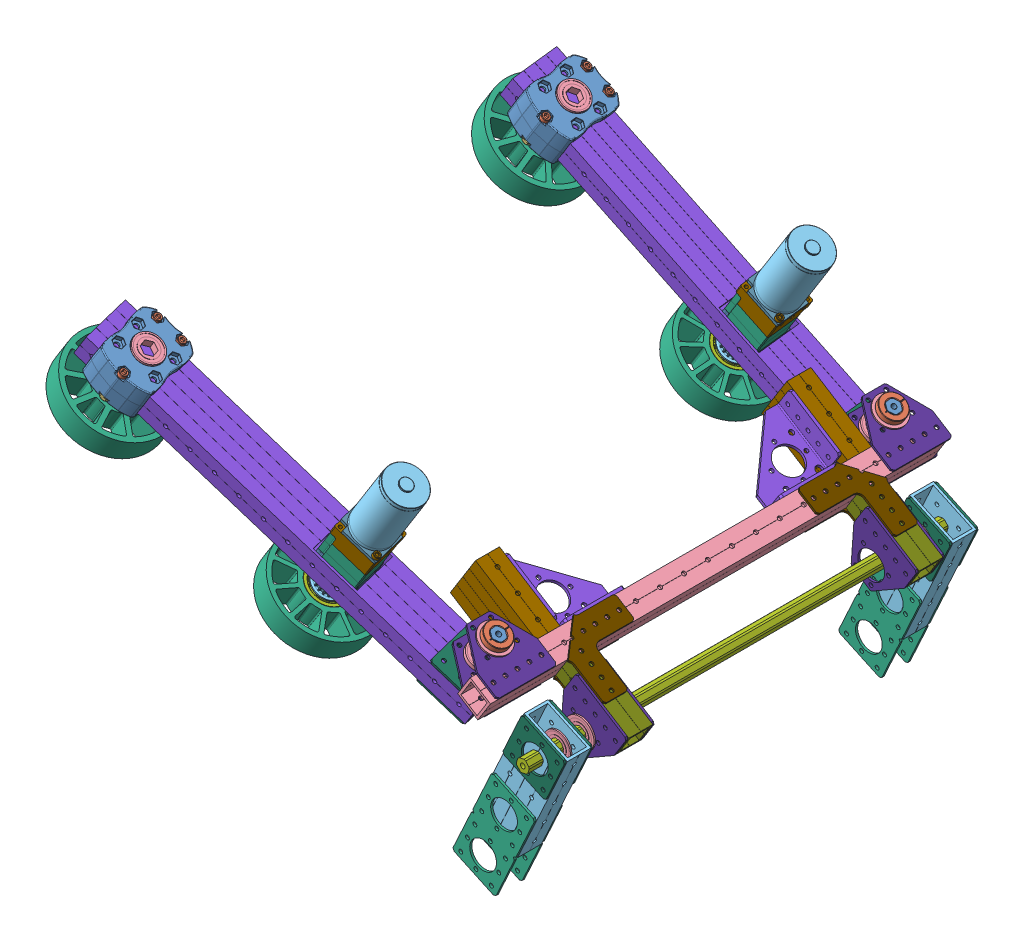
SolidWorks assembly Intake, configuration Default. Lengths in mm.
Overall size (503.07 503.81 614.92).
182 component instances, 45 part files, 124 mates.
Components (placement in the parent):
- Arm-3: Arm [Default] at (-23.47 463.3123 635.721) x (-0.531639 -0.846966 -0.002975) z (-0.831467 0.521235 0.192294) size (182.24 117.43 425.71)
  - PlasticBerringClamps-1: PlasticBerringClamps [Default] at (91.1348 153.644 -362.2083) size (41.46 73.98 53.68)
    - 217-4155-001 Rev6-1: 217-4155-001 Rev6 [Default] at (-3.3739 45.2343 730.1325) x (0 0 -1) z (1 0 0) size (53.68 71 22.06)
    - 217-4155-001 Rev6-2: 217-4155-001 Rev6 [Default] at (-3.3739 45.2343 730.1325) x (0 0 1) z (-1 0 0) size (53.68 71 22.06)
    - 217-4155-003 Rev1_SSA1032-1375ZB-1: 217-4155-003 Rev1_SSA1032-1375ZB [Default] at (-18.0739 75.1843 730.1325) x (0 1 0) z (0 0 1) size (7.87 39.75 7.87)
    - 217-4155-003 Rev1_SSA1032-1375ZB-2: 217-4155-003 Rev1_SSA1032-1375ZB [Default] at (-18.0739 15.2843 717.4325) x (0 1 0) z (0 0 1) size (7.87 39.75 7.87)
    - 217-4155-003 Rev1_SSA1032-1375ZB-3: 217-4155-003 Rev1_SSA1032-1375ZB [Default] at (-18.0739 15.2843 742.8325) x (0 1 0) z (0 0 1) size (7.87 39.75 7.87)
    - 217-4155-002 Rev2_NNY1032-ZC-1: 217-4155-002 Rev2_NNY1032-ZC [Default] at (11.3261 15.2843 717.4325) x (0 -0.5 -0.866025) z (1 0 0) size (9.39 10.84 4.45)
    - 217-4155-002 Rev2_NNY1032-ZC-2: 217-4155-002 Rev2_NNY1032-ZC [Default] at (11.3261 15.2843 742.8325) x (0 -0.5 -0.866025) z (1 0 0) size (9.39 10.84 4.45)
    - 217-4155-002 Rev2_NNY1032-ZC-3: 217-4155-002 Rev2_NNY1032-ZC [Default] at (11.3261 75.1843 730.1325) x (0 0.5 -0.866025) z (1 0 0) size (9.39 10.84 4.45)
    - FlangedBerring-1: FlangedBerring [Default] at (17.3541 43.6343 730.1325) x (0 0.579557 0.814931) z (0 -0.814931 0.579557) size (31.12 7.94 31.12)
    - FlangedBerring-2: FlangedBerring [Default] at (-24.1019 43.6343 730.1325) x (0 0.415973 -0.909377) z (0 -0.909377 -0.415973) size (31.12 7.94 31.12)
  - 18tSproket-1: 18tSproket [Default] at (115.7389 197.2783 367.9242) x (0 0.046999 0.998895) z (1 0 0) size (32 32 14.5)
  - 18tSproket-2: 18tSproket [Default] at (115.7389 199.082 150.8743) x (0 0.078751 0.996894) z (-1 0 0) size (32 32 14.5)
  - 4inTractionWheels-1: 4inTractionWheels [Default] at (129.7369 180.6221 368.9515) x (0 -0.985371 -0.170422) z (1 0 0) size (101.6 101.6 25.74)
    - 4IN Compliant Wheel FINAL Overmold-1: 4IN Compliant Wheel FINAL Overmold [Default] at (-16.2374 3.8509 18.652) size (101.6 101.6 25.74)
    - 2in Wheel Intergrated 0500 HEX Hub-1: 2in Wheel Intergrated 0500 HEX Hub [Default] at (-16.2374 3.8509 5.952) x (-1 0 0) z (0 0 -1) size (41.91 41.91 25.4)
  - 4inTractionWheels-2: 4inTractionWheels [Default] at (141.6409 215.6464 152.9003) x (0 0.993829 -0.110924) z (-1 0 0) size (101.6 101.6 25.74)
    - 4IN Compliant Wheel FINAL Overmold-1: 4IN Compliant Wheel FINAL Overmold [Default] at (-16.2374 3.8509 18.652) size (101.6 101.6 25.74)
    - 2in Wheel Intergrated 0500 HEX Hub-1: 2in Wheel Intergrated 0500 HEX Hub [Default] at (-16.2374 3.8509 5.952) x (-1 0 0) z (0 0 -1) size (41.91 41.91 25.4)
  - 1x2x16StockSlotted-1: 1x2x16StockSlotted [12] at (87.8609 198.8783 750.2323) x (-1 0 0) z (0 0 -1) size (25.4 50.8 406.4)
  - BagMotor2StageGearBox-1: BagMotor2StageGearBox [Default] at (46.4959 199.082 150.8743) x (0 0 1) z (-1 0 0) size (49.3 49.3 173.58)
    - 217-2625-001 Rev1-1: 217-2625-001 Rev1 [Default] at origin size (42 42 18)
    - 217-2625-002 Rev1-1: 217-2625-002 Rev1 [Default] at (0 0 -29.4) size (42 42 17.13)
    - 217-2625-003 Rev1-1: 217-2625-003 Rev1 [Default] at (0 0 -43.6478) x (0.966651 -0.256095 0) z (0 0 -1) size (17 17 64.12)
    - 217-2625-009 Rev1-1: 217-2625-009 Rev1 [Default] at (0 0 -3.48) x (-0.609619 0.792694 0) z (0 0 -1) size (18 18 13)
    - 217-2625-100-1: 217-2625-100 [Default] at (0 0 -18.8454) x (0.784104 -0.62063 0) z (0 0 1) size (39.26 38.9 12.7)
      - 217-2625-008 Rev1-1: 217-2625-008 Rev1 [Default] at origin size (34.7 34.7 4.7)
      - 217-2625-010 Rev1-1: 217-2625-010 Rev1 [Default] at (0 10.193 3.65) x (0.999813 0.019336 0) z (0 0 1) size (4 4 12)
      - 217-2625-010 Rev1-2: 217-2625-010 Rev1 [Default] at (8.691 -5.3258 3.65) size (4 4 12)
      - 217-2625-010 Rev1-3: 217-2625-010 Rev1 [Default] at (-8.691 -5.3258 3.65) size (4 4 12)
      - 217-2625-005 Rev1_Planet_Revolving_Follower01-1: 217-2625-005 Rev1_Planet_Revolving_Follower01 [Default] at (8.691 -5.3258 6.35) x (0.932816 0.360354 0) z (0 0 1) size (16.91 16.92 8)
      - 217-2625-005 Rev1_Planet_Revolving_Follower01-2: 217-2625-005 Rev1_Planet_Revolving_Follower01 [Default] at (-8.691 -5.3258 6.35) x (-0.932788 -0.360426 0) z (0 0 1) size (16.91 16.92 8)
      - 217-2625-005 Rev1_Planet_Revolving_Follower01-3: 217-2625-005 Rev1_Planet_Revolving_Follower01 [Default] at (0 10.193 6.35) x (0.893583 0.448898 0) z (0 0 1) size (16.91 16.92 8)
    - 217-2625-007 Rev1_Sun_Driver01-1: 217-2625-007 Rev1_Sun_Driver01 [Default] at (0 0 -11.5575) x (0.564419 -0.825488 0) z (0 0 1) size (14.49 14.49 12.72)
    - 217-2742-1: 217-2742 [Default] at (0 0 -51.4002) x (0 0 1) z (-0.997393 0.072165 0) size (7 28 28)
    - 217-2742-2: 217-2742 [Default] at (0 0 -43.1002) x (0 0 1) z (-1 0 0) size (7 28 28)
    - 217-2741-1: 217-2741 [Default] at (0 0 -7) x (0 0 1) z (-0.951311 0.308231 0) size (5 26 26)
    - TRUARC-MSH-15_98541A410-1: TRUARC-MSH-15_98541A410 [Default] at (0 0 -35.4954) x (0 0 -1) z (0.980859 -0.194721 0) size (1 19.6 17.4)
    - SPRGW0856-1102-012_9714K62-1: SPRGW0856-1102-012_9714K62 [Default] at (0 0 -44.1002) x (-0.695225 0.718792 0) z (-0.718792 -0.695225 0) size (29.09 5.11 30.79)
    - SSS1032-0125ZB_94105A824-1: SSS1032-0125ZB_94105A824 [Default] at (5.4759 4.2112 1.995) x (-0.605001 0.78669 -0.122849) z (0.792694 0.609619 0) size (4.83 4.84 3.3)
    - TRUARC-5103-68_97414A675_grv-1: TRUARC-5103-68_97414A675_grv [Default] at (1.1965 0.0349 -1.3834) x (0 0 -1) z (-0.029125 0.999576 0) size (1.07 15.49 20.19)
    - 217-3351-1: 217-3351 [Default] at (0 0 10.675) x (0 -1 0) z (0 0 -1) size (40.4 40.4 81.5)
    - 217-2816-001 Rev1-1: 217-2816-001 Rev1 [Default] at (0 0 -29.55) x (1 0 0) z (0 0 -1) size (42 42 14.5)
    - SSA_SSA0832-1750ZC-1: SSA_SSA0832-1750ZC [Default] at (-17.5 17.5 -47.261) x (-0.769034 -0.639207 0) z (0.639207 -0.769034 0) size (6.73 48.51 6.73)
    - SSA_SSA0832-1750ZC-2: SSA_SSA0832-1750ZC [Default] at (17.5 -17.5 -47.261) x (0.162252 0.986749 0) z (-0.986749 0.162252 0) size (6.73 48.51 6.73)
    - 217-2625-011 Rev1-1: 217-2625-011 Rev1 [Default] at (0 0 1.37) x (-0.792694 -0.609619 0) z (-0.609619 0.792694 0) size (8.01 7.5 7.94)
    - SSA_SSA0832-0500ZC-1: SSA_SSA0832-0500ZC [Default] at (-17.5 17.5 10.675) x (0.592766 0.805375 0) z (0.805375 -0.592766 0) size (6.73 16.76 6.73)
    - SSA_SSA0832-0500ZC-2: SSA_SSA0832-0500ZC [Default] at (17.5 -17.5 10.675) x (-0.592766 -0.805375 0) z (-0.805375 0.592766 0) size (6.73 16.76 6.73)
    - SSHCM004_SSHCM004070010C-1: SSHCM004_SSHCM004070010C [Default] at (0 -12.5 7.5) x (-0.451598 -0.892221 0) z (0.892221 -0.451598 0) size (7 14 7)
    - SSHCM004_SSHCM004070010C-2: SSHCM004_SSHCM004070010C [Default] at (0 12.5 7.5) x (-0.447517 -0.894275 0) z (0.894275 -0.447517 0) size (7 14 7)
    - 217-2816-001 Rev1-2: 217-2816-001 Rev1 [Default] at (0 0 -16.85) x (1 0 0) z (0 0 -1) size (42 42 14.5)
    - 217-2818 Rev1-1: 217-2818 Rev1 [Default] at (0 0 -31.5454) size (49.07 49.07 17.4)
      - 217-2725-001 Rev1_24t Sun-1: 217-2725-001 Rev1_24t Sun [Default] at (0 0 8.7) size (14.45 14.45 12.7)
      - 217-2725-002 Rev1_24t Planet-1: 217-2725-002 Rev1_24t Planet [Default] at (-12.089 0 6.35) x (-0.130526 0.991445 0) z (0 0 -1) size (13.17 13.15 8)
      - 217-2724-002 Rev1-1: 217-2724-002 Rev1 [Default] x (0.707107 -0.707107 0) z (0 0 -1) size (34.7 34.7 4.7)
      - 217-2625-010 Rev1-1: 217-2625-010 Rev1 [Default] at (-12.089 0 3.65) x (0.971612 -0.236582 0) z (0 0 1) size (4 4 12)
      - 217-2725-002 Rev1_24t Planet-2: 217-2725-002 Rev1_24t Planet [Default] at (0 -12.089 6.35) x (-0.991445 -0.130526 0) z (0 0 -1) size (13.17 13.15 8)
      - 217-2725-002 Rev1_24t Planet-3: 217-2725-002 Rev1_24t Planet [Default] at (12.089 0 6.35) x (0.130526 -0.991445 0) z (0 0 -1) size (13.17 13.15 8)
      - 217-2725-002 Rev1_24t Planet-4: 217-2725-002 Rev1_24t Planet [Default] at (0 12.089 6.35) x (0.991445 0.130526 0) z (0 0 -1) size (13.17 13.15 8)
      - 217-2625-010 Rev1-2: 217-2625-010 Rev1 [Default] at (0 -12.089 3.65) x (0.236582 0.971612 0) z (0 0 1) size (4 4 12)
      - 217-2625-010 Rev1-3: 217-2625-010 Rev1 [Default] at (12.089 0 3.65) x (-0.971612 0.236582 0) z (0 0 1) size (4 4 12)
      - 217-2625-010 Rev1-4: 217-2625-010 Rev1 [Default] at (0 12.089 3.65) x (-0.236582 -0.971612 0) z (0 0 1) size (4 4 12)
    - 217-2822-003 Rev4-1: 217-2822-003 Rev4 [Default] at (0 0 9) x (0 -1 0) z (0 0 1) size (42 42 4.8)
  - FaceBerringMountGussetHalved-1: FaceBerringMountGussetHalved [Default] at (72.8749 224.1513 26.2053) x (0 1 0) z (1 0 0) size (50.67 50.55 2.29)
  - FaceBerringMountGussetHalved-3: FaceBerringMountGussetHalved [Default] at (100.5609 198.7513 0.9323) x (0 0 -1) z (1 0 0) size (50.67 50.55 2.29)
  - FlangedBerring-1: FlangedBerring [Default] at (96.4969 198.7513 27.6404) x (0 0.415973 -0.909377) z (0 -0.909377 -0.415973) size (31.12 7.94 31.12)
  - FlangedBerring-2: FlangedBerring [Default] at (79.2249 197.4432 26.2053) x (0 -0.140437 0.99009) z (0 -0.99009 -0.140437) size (31.12 7.94 31.12)
- 1x1x3Stock-3: 1x1x3Stock [Default] at (630.636 -4.873 778.4629) x (-0.002909 -0.001687 0.999994) z (0.846966 -0.531645 0.001567) size (25.4 25.4 76.2)
- SideBerringGusset-2: SideBerringGusset [Default] at (-31.1533 428.0283 834.4183) x (0.002909 0.001687 -0.999994) z (-0.531639 -0.846966 -0.002975) size (63.5 61.91 2.29)
- SideBerringGusset-3: SideBerringGusset [Default] at (-47.0875 402.643 834.3291) x (-0.002909 -0.001687 0.999994) z (0.531639 0.846966 0.002975) size (63.5 61.91 2.29)
- FlangedBerring-11: FlangedBerring [Default] at (-34.5292 422.6501 834.3994) x (0.844713 -0.529962 -0.07483) z (0.061802 -0.042296 0.997192) size (31.12 7.94 31.12)
- FlangedBerring-12: FlangedBerring [Default] at (-43.7116 408.0213 834.348) x (-0.292306 0.180181 0.939198) z (0.794932 -0.500184 0.343364) size (31.12 7.94 31.12)
- SideBerringGusset-4: SideBerringGusset [Default] at (19.3994 346.1992 454.4895) x (0.846966 -0.531645 0.001567) z (-0.002909 -0.001687 0.999994) size (63.5 61.91 2.29)
- FlangedBerring-13: FlangedBerring [Default] at (19.3809 346.1885 460.8395) x (0.999707 0.024044 0.002949) z (-0.024049 0.999709 0.001616) size (31.12 7.94 31.12)
- SideBerringGusset-5: SideBerringGusset [Default] at (18.4974 345.6762 764.5734) x (-0.846966 0.531645 -0.001567) z (0.002909 0.001687 -0.999994) size (63.5 61.91 2.29)
- SideBerringGusset-6: SideBerringGusset [Default] at (18.4235 345.6333 789.9733) x (0.846966 -0.531645 0.001567) z (-0.002909 -0.001687 0.999994) size (63.5 61.91 2.29)
- SideBerringGusset-7: SideBerringGusset [Default] at (19.3188 346.1525 482.1754) x (0.846966 -0.531645 0.001567) z (-0.002909 -0.001687 0.999994) size (63.5 61.91 2.29)
- FlangedBerring-15: FlangedBerring [Default] at (18.4353 345.6402 785.9093) x (-0.001685 0.999997 0.001682) z (0.999994 0.00168 0.002912) size (31.12 7.94 31.12)
- 1x1x3Stock-5: 1x1x3Stock [Default] at (631.5313 -4.3539 470.665) x (-0.002909 -0.001687 0.999994) z (0.846966 -0.531645 0.001567) size (25.4 25.4 76.2)
- PlusGussetHalved-7: PlusGussetHalved [Default] at (-22.7192 387.5477 777.2242) x (-0.846966 0.531645 -0.001567) z (0.531639 0.846966 0.002975) size (71.47 72 2.29)
- PlusGussetHalved-8: PlusGussetHalved [Default] at (-7.1049 411.5159 469.5087) x (0.002909 0.001687 -0.999994) z (0.531639 0.846966 0.002975) size (71.47 72 2.29)
- PlusGussetHalved-9: PlusGussetHalved [Default] at (-21.8239 388.0668 469.4263) x (0.002909 0.001687 -0.999994) z (0.531639 0.846966 0.002975) size (71.47 72 2.29)
- SideBerringGusset-8: SideBerringGusset [Default] at (-45.8684 403.3499 415.2315) x (-0.002909 -0.001687 0.999994) z (0.531639 0.846966 0.002975) size (63.5 61.91 2.29)
- SideBerringGusset-9: SideBerringGusset [Default] at (-31.1494 426.799 415.3138) x (-0.002909 -0.001687 0.999994) z (0.531639 0.846966 0.002975) size (63.5 61.91 2.29)
- FlangedBerring-19: FlangedBerring [Default] at (-33.31 423.3569 415.3017) x (0.837705 -0.525302 -0.149357) z (0.124937 -0.081896 0.988779) size (31.12 7.94 31.12)
- FlangedBerring-21: FlangedBerring [Default] at (-42.4925 408.7281 415.2504) x (-0.844713 0.529962 0.07483) z (0.061802 -0.042296 0.997192) size (31.12 7.94 31.12)
- HexShaft3.5in-1: HexShaft3.5in [Default] at (48.5558 553.7791 415.7599) x (-0.061802 0.042296 -0.997192) z (0.531639 0.846966 0.002975) size (13.74 12.75 88.9)
- ShaftCollar-1: ShaftCollar [Default] at (-27.4022 432.7688 415.3348) x (-0.061802 0.042296 -0.997192) z (0.531639 0.846966 0.002975) size (25.39 25.4 7.82)
- 1_4inSpacer-1: 1_4inSpacer [Default] at (-48.4003 399.3162 415.2173) x (-0.061802 0.042296 -0.997192) z (0.531639 0.846966 0.002975) size (19.5 19.5 6.35)
- ShaftCollar-2: ShaftCollar [Default] at (-70.5169 366.5607 416.5259) x (-0.061802 0.042296 -0.997192) z (0.531639 0.846966 0.002975) size (25.39 25.4 7.82)
- Arm-5: Arm [Default] at (-4.0746 452.6105 216.4592) x (-0.531639 -0.846966 -0.002975) z (-0.843997 0.529475 0.085594) size (182.24 117.43 425.71)
  - PlasticBerringClamps-1: PlasticBerringClamps [Default] at (91.1348 153.644 -362.2083) size (41.46 73.98 53.68)
    - 217-4155-001 Rev6-1: 217-4155-001 Rev6 [Default] at (-3.3739 45.2343 730.1325) x (0 0 -1) z (1 0 0) size (53.68 71 22.06)
    - 217-4155-001 Rev6-2: 217-4155-001 Rev6 [Default] at (-3.3739 45.2343 730.1325) x (0 0 1) z (-1 0 0) size (53.68 71 22.06)
    - 217-4155-003 Rev1_SSA1032-1375ZB-1: 217-4155-003 Rev1_SSA1032-1375ZB [Default] at (-18.0739 75.1843 730.1325) x (0 1 0) z (0 0 1) size (7.87 39.75 7.87)
    - 217-4155-003 Rev1_SSA1032-1375ZB-2: 217-4155-003 Rev1_SSA1032-1375ZB [Default] at (-18.0739 15.2843 717.4325) x (0 1 0) z (0 0 1) size (7.87 39.75 7.87)
    - 217-4155-003 Rev1_SSA1032-1375ZB-3: 217-4155-003 Rev1_SSA1032-1375ZB [Default] at (-18.0739 15.2843 742.8325) x (0 1 0) z (0 0 1) size (7.87 39.75 7.87)
    - 217-4155-002 Rev2_NNY1032-ZC-1: 217-4155-002 Rev2_NNY1032-ZC [Default] at (11.3261 15.2843 717.4325) x (0 -0.5 -0.866025) z (1 0 0) size (9.39 10.84 4.45)
    - 217-4155-002 Rev2_NNY1032-ZC-2: 217-4155-002 Rev2_NNY1032-ZC [Default] at (11.3261 15.2843 742.8325) x (0 -0.5 -0.866025) z (1 0 0) size (9.39 10.84 4.45)
    - 217-4155-002 Rev2_NNY1032-ZC-3: 217-4155-002 Rev2_NNY1032-ZC [Default] at (11.3261 75.1843 730.1325) x (0 0.5 -0.866025) z (1 0 0) size (9.39 10.84 4.45)
    - FlangedBerring-1: FlangedBerring [Default] at (17.3541 43.6343 730.1325) x (0 0.579557 0.814931) z (0 -0.814931 0.579557) size (31.12 7.94 31.12)
    - FlangedBerring-2: FlangedBerring [Default] at (-24.1019 43.6343 730.1325) x (0 0.415973 -0.909377) z (0 -0.909377 -0.415973) size (31.12 7.94 31.12)
  - 18tSproket-1: 18tSproket [Default] at (115.7389 197.2783 367.9242) x (0 0.046999 0.998895) z (1 0 0) size (32 32 14.5)
  - 18tSproket-2: 18tSproket [Default] at (115.7389 199.082 150.8743) x (0 0.078751 0.996894) z (-1 0 0) size (32 32 14.5)
  - 4inTractionWheels-1: 4inTractionWheels [Default] at (129.7369 180.6221 368.9515) x (0 -0.985371 -0.170422) z (1 0 0) size (101.6 101.6 25.74)
    - 4IN Compliant Wheel FINAL Overmold-1: 4IN Compliant Wheel FINAL Overmold [Default] at (-16.2374 3.8509 18.652) size (101.6 101.6 25.74)
    - 2in Wheel Intergrated 0500 HEX Hub-1: 2in Wheel Intergrated 0500 HEX Hub [Default] at (-16.2374 3.8509 5.952) x (-1 0 0) z (0 0 -1) size (41.91 41.91 25.4)
  - 4inTractionWheels-2: 4inTractionWheels [Default] at (141.6409 215.6464 152.9003) x (0 0.993829 -0.110924) z (-1 0 0) size (101.6 101.6 25.74)
    - 4IN Compliant Wheel FINAL Overmold-1: 4IN Compliant Wheel FINAL Overmold [Default] at (-16.2374 3.8509 18.652) size (101.6 101.6 25.74)
    - 2in Wheel Intergrated 0500 HEX Hub-1: 2in Wheel Intergrated 0500 HEX Hub [Default] at (-16.2374 3.8509 5.952) x (-1 0 0) z (0 0 -1) size (41.91 41.91 25.4)
  - 1x2x16StockSlotted-1: 1x2x16StockSlotted [12] at (87.8609 198.8783 750.2323) x (-1 0 0) z (0 0 -1) size (25.4 50.8 406.4)
  - BagMotor2StageGearBox-1: BagMotor2StageGearBox [Default] at (46.4959 199.082 150.8743) x (0 0 1) z (-1 0 0) size (49.3 49.3 173.58)
    - 217-2625-001 Rev1-1: 217-2625-001 Rev1 [Default] at origin size (42 42 18)
    - 217-2625-002 Rev1-1: 217-2625-002 Rev1 [Default] at (0 0 -29.4) size (42 42 17.13)
    - 217-2625-003 Rev1-1: 217-2625-003 Rev1 [Default] at (0 0 -43.6478) x (0.966651 -0.256095 0) z (0 0 -1) size (17 17 64.12)
    - 217-2625-009 Rev1-1: 217-2625-009 Rev1 [Default] at (0 0 -3.48) x (-0.609619 0.792694 0) z (0 0 -1) size (18 18 13)
    - 217-2625-100-1: 217-2625-100 [Default] at (0 0 -18.8454) x (0.784104 -0.62063 0) z (0 0 1) size (39.26 38.9 12.7)
      - 217-2625-008 Rev1-1: 217-2625-008 Rev1 [Default] at origin size (34.7 34.7 4.7)
      - 217-2625-010 Rev1-1: 217-2625-010 Rev1 [Default] at (0 10.193 3.65) x (0.999813 0.019336 0) z (0 0 1) size (4 4 12)
      - 217-2625-010 Rev1-2: 217-2625-010 Rev1 [Default] at (8.691 -5.3258 3.65) size (4 4 12)
      - 217-2625-010 Rev1-3: 217-2625-010 Rev1 [Default] at (-8.691 -5.3258 3.65) size (4 4 12)
      - 217-2625-005 Rev1_Planet_Revolving_Follower01-1: 217-2625-005 Rev1_Planet_Revolving_Follower01 [Default] at (8.691 -5.3258 6.35) x (0.932816 0.360354 0) z (0 0 1) size (16.91 16.92 8)
      - 217-2625-005 Rev1_Planet_Revolving_Follower01-2: 217-2625-005 Rev1_Planet_Revolving_Follower01 [Default] at (-8.691 -5.3258 6.35) x (-0.932788 -0.360426 0) z (0 0 1) size (16.91 16.92 8)
      - 217-2625-005 Rev1_Planet_Revolving_Follower01-3: 217-2625-005 Rev1_Planet_Revolving_Follower01 [Default] at (0 10.193 6.35) x (0.893583 0.448898 0) z (0 0 1) size (16.91 16.92 8)
    - 217-2625-007 Rev1_Sun_Driver01-1: 217-2625-007 Rev1_Sun_Driver01 [Default] at (0 0 -11.5575) x (0.564419 -0.825488 0) z (0 0 1) size (14.49 14.49 12.72)
    - 217-2742-1: 217-2742 [Default] at (0 0 -51.4002) x (0 0 1) z (-0.997393 0.072165 0) size (7 28 28)
    - 217-2742-2: 217-2742 [Default] at (0 0 -43.1002) x (0 0 1) z (-1 0 0) size (7 28 28)
    - 217-2741-1: 217-2741 [Default] at (0 0 -7) x (0 0 1) z (-0.951311 0.308231 0) size (5 26 26)
    - TRUARC-MSH-15_98541A410-1: TRUARC-MSH-15_98541A410 [Default] at (0 0 -35.4954) x (0 0 -1) z (0.980859 -0.194721 0) size (1 19.6 17.4)
    - SPRGW0856-1102-012_9714K62-1: SPRGW0856-1102-012_9714K62 [Default] at (0 0 -44.1002) x (-0.695225 0.718792 0) z (-0.718792 -0.695225 0) size (29.09 5.11 30.79)
    - SSS1032-0125ZB_94105A824-1: SSS1032-0125ZB_94105A824 [Default] at (5.4759 4.2112 1.995) x (-0.605001 0.78669 -0.122849) z (0.792694 0.609619 0) size (4.83 4.84 3.3)
    - TRUARC-5103-68_97414A675_grv-1: TRUARC-5103-68_97414A675_grv [Default] at (1.1965 0.0349 -1.3834) x (0 0 -1) z (-0.029125 0.999576 0) size (1.07 15.49 20.19)
    - 217-3351-1: 217-3351 [Default] at (0 0 10.675) x (0 -1 0) z (0 0 -1) size (40.4 40.4 81.5)
    - 217-2816-001 Rev1-1: 217-2816-001 Rev1 [Default] at (0 0 -29.55) x (1 0 0) z (0 0 -1) size (42 42 14.5)
    - SSA_SSA0832-1750ZC-1: SSA_SSA0832-1750ZC [Default] at (-17.5 17.5 -47.261) x (-0.769034 -0.639207 0) z (0.639207 -0.769034 0) size (6.73 48.51 6.73)
    - SSA_SSA0832-1750ZC-2: SSA_SSA0832-1750ZC [Default] at (17.5 -17.5 -47.261) x (0.162252 0.986749 0) z (-0.986749 0.162252 0) size (6.73 48.51 6.73)
    - 217-2625-011 Rev1-1: 217-2625-011 Rev1 [Default] at (0 0 1.37) x (-0.792694 -0.609619 0) z (-0.609619 0.792694 0) size (8.01 7.5 7.94)
    - SSA_SSA0832-0500ZC-1: SSA_SSA0832-0500ZC [Default] at (-17.5 17.5 10.675) x (0.592766 0.805375 0) z (0.805375 -0.592766 0) size (6.73 16.76 6.73)
    - SSA_SSA0832-0500ZC-2: SSA_SSA0832-0500ZC [Default] at (17.5 -17.5 10.675) x (-0.592766 -0.805375 0) z (-0.805375 0.592766 0) size (6.73 16.76 6.73)
    - SSHCM004_SSHCM004070010C-1: SSHCM004_SSHCM004070010C [Default] at (0 -12.5 7.5) x (-0.451598 -0.892221 0) z (0.892221 -0.451598 0) size (7 14 7)
    - SSHCM004_SSHCM004070010C-2: SSHCM004_SSHCM004070010C [Default] at (0 12.5 7.5) x (-0.447517 -0.894275 0) z (0.894275 -0.447517 0) size (7 14 7)
    - 217-2816-001 Rev1-2: 217-2816-001 Rev1 [Default] at (0 0 -16.85) x (1 0 0) z (0 0 -1) size (42 42 14.5)
    - 217-2818 Rev1-1: 217-2818 Rev1 [Default] at (0 0 -31.5454) size (49.07 49.07 17.4)
      - 217-2725-001 Rev1_24t Sun-1: 217-2725-001 Rev1_24t Sun [Default] at (0 0 8.7) size (14.45 14.45 12.7)
      - 217-2725-002 Rev1_24t Planet-1: 217-2725-002 Rev1_24t Planet [Default] at (-12.089 0 6.35) x (-0.130526 0.991445 0) z (0 0 -1) size (13.17 13.15 8)
      - 217-2724-002 Rev1-1: 217-2724-002 Rev1 [Default] x (0.707107 -0.707107 0) z (0 0 -1) size (34.7 34.7 4.7)
      - 217-2625-010 Rev1-1: 217-2625-010 Rev1 [Default] at (-12.089 0 3.65) x (0.971612 -0.236582 0) z (0 0 1) size (4 4 12)
      - 217-2725-002 Rev1_24t Planet-2: 217-2725-002 Rev1_24t Planet [Default] at (0 -12.089 6.35) x (-0.991445 -0.130526 0) z (0 0 -1) size (13.17 13.15 8)
      - 217-2725-002 Rev1_24t Planet-3: 217-2725-002 Rev1_24t Planet [Default] at (12.089 0 6.35) x (0.130526 -0.991445 0) z (0 0 -1) size (13.17 13.15 8)
      - 217-2725-002 Rev1_24t Planet-4: 217-2725-002 Rev1_24t Planet [Default] at (0 12.089 6.35) x (0.991445 0.130526 0) z (0 0 -1) size (13.17 13.15 8)
      - 217-2625-010 Rev1-2: 217-2625-010 Rev1 [Default] at (0 -12.089 3.65) x (0.236582 0.971612 0) z (0 0 1) size (4 4 12)
      - 217-2625-010 Rev1-3: 217-2625-010 Rev1 [Default] at (12.089 0 3.65) x (-0.971612 0.236582 0) z (0 0 1) size (4 4 12)
      - 217-2625-010 Rev1-4: 217-2625-010 Rev1 [Default] at (0 12.089 3.65) x (-0.236582 -0.971612 0) z (0 0 1) size (4 4 12)
    - 217-2822-003 Rev4-1: 217-2822-003 Rev4 [Default] at (0 0 9) x (0 -1 0) z (0 0 1) size (42 42 4.8)
  - FaceBerringMountGussetHalved-1: FaceBerringMountGussetHalved [Default] at (72.8749 224.1513 26.2053) x (0 1 0) z (1 0 0) size (50.67 50.55 2.29)
  - FaceBerringMountGussetHalved-3: FaceBerringMountGussetHalved [Default] at (100.5609 198.7513 0.9323) x (0 0 -1) z (1 0 0) size (50.67 50.55 2.29)
  - FlangedBerring-1: FlangedBerring [Default] at (96.4969 198.7513 27.6404) x (0 0.415973 -0.909377) z (0 -0.909377 -0.415973) size (31.12 7.94 31.12)
  - FlangedBerring-2: FlangedBerring [Default] at (79.2249 197.4432 26.2053) x (0 -0.140437 0.99009) z (0 -0.99009 -0.140437) size (31.12 7.94 31.12)
- ShaftCollar-3: ShaftCollar [Default] at (-28.6213 432.062 834.4324) x (-0.061802 0.042296 -0.997192) z (0.531639 0.846966 0.002975) size (25.39 25.4 7.82)
- HexShaft3.5in-2: HexShaft3.5in [Default] at (47.3366 553.0722 834.8575) x (-0.061802 0.042296 -0.997192) z (0.531639 0.846966 0.002975) size (13.74 12.75 88.9)
- ShaftCollar-5: ShaftCollar [Default] at (-71.5998 365.7678 835.7571) x (-0.061802 0.042296 -0.997192) z (0.531639 0.846966 0.002975) size (25.39 25.4 7.82)
- 1_4inSpacer-3: 1_4inSpacer [Default] at (-49.6195 398.6094 834.3149) x (-0.061802 0.042296 -0.997192) z (0.531639 0.846966 0.002975) size (19.5 19.5 6.35)
- 1x1x19Stock-2: 1x1x19Stock [Default] at (-15.805 399.6298 1139.2167) x (-0.531639 -0.846966 -0.002975) z (-0.002909 -0.001687 0.999994) size (25.4 25.4 482.6)
- 1x2x5HoledStock-2: 1x2x5HoledStock [12] at (-282.9319 -311.5782 417.9081) x (0.002909 0.001687 -0.999994) z (0.419348 0.907821 0.002751) size (25.4 50.8 127)
- FaceBerringMountGussetHalved-1: FaceBerringMountGussetHalved [Default] at (43.7092 335.036 432.6489) x (0.907821 -0.419354 0.001934) z (-0.002909 -0.001687 0.999994) size (50.67 50.55 2.29)
- FaceBerringMountGussetHalved-2: FaceBerringMountGussetHalved [Default] at (43.7896 335.0825 405.0393) x (0.907821 -0.419354 0.001934) z (-0.002909 -0.001687 0.999994) size (50.67 50.55 2.29)
- FaceBerringMountGusset-10: FaceBerringMountGusset [Default] at (-21.9464 253.169 432.3199) x (-0.419348 -0.907821 -0.002751) z (-0.002909 -0.001687 0.999994) size (101.35 50.55 2.29)
- FaceBerringMountGusset-11: FaceBerringMountGusset [Default] at (-21.8659 253.2157 404.634) x (-0.419348 -0.907821 -0.002751) z (-0.002909 -0.001687 0.999994) size (101.35 50.55 2.29)
- FlangedBerring-22: FlangedBerring [Default] at (19.4749 346.2429 428.5333) x (-0.001685 0.999997 0.001682) z (0.999994 0.00168 0.002912) size (31.12 7.94 31.12)
- FlangedBerring-23: FlangedBerring [Default] at (18.3429 345.5866 817.6591) x (-0.255661 0.966766 0.000887) z (-0.966762 -0.255657 -0.003243) size (31.12 7.94 31.12)
- FaceBerringMountGussetHalved-5: FaceBerringMountGussetHalved [Default] at (-5.9717 356.7471 841.1531) x (-0.907821 0.419354 -0.001934) z (0.002909 0.001687 -0.999994) size (50.67 50.55 2.29)
- FaceBerringMountGusset-12: FaceBerringMountGusset [Default] at (-25.6603 253.7301 813.3122) x (-0.419348 -0.907821 -0.002751) z (0.002909 0.001687 -0.999994) size (101.35 50.55 2.29)
- FaceBerringMountGusset-13: FaceBerringMountGusset [Default] at (-25.7409 253.6834 840.998) x (-0.419348 -0.907821 -0.002751) z (0.002909 0.001687 -0.999994) size (101.35 50.55 2.29)
- FaceBerringMountGussetHalved-6: FaceBerringMountGussetHalved [Default] at (-5.8914 356.7936 813.5435) x (-0.907821 0.419354 -0.001934) z (0.002909 0.001687 -0.999994) size (50.67 50.55 2.29)
- 1x2x5HoledStock-4: 1x2x5HoledStock [12] at (-286.4891 -311.1665 824.3007) x (-0.002909 -0.001687 0.999994) z (0.419348 0.907821 0.002751) size (25.4 50.8 127)
- HexShaft-3: HexShaft [Default] at (18.9025 345.9111 625.306) x (0.313178 0.949691 0.002513) z (-0.002909 -0.001687 0.999994) size (13.74 12.75 457.2)
- PlusGussetHalved-12: PlusGussetHalved [Default] at (-8.0003 410.9968 777.3066) x (-0.846966 0.531645 -0.001567) z (0.531639 0.846966 0.002975) size (71.47 72 2.29)
- CornerGusset-1: CornerGusset [Default] at (-32.2604 396.2357 777.2111) x (0.002909 0.001687 -0.999994) z (0.531639 0.846966 0.002975) size (69.72 69.72 25.4)
- CornerGusset-2: CornerGusset [Default] at (-31.3737 396.7498 472.4128) x (-0.846966 0.531645 -0.001567) z (0.531639 0.846966 0.002975) size (69.72 69.72 25.4)
- 1x2x3Stock-1: 1x2x3Stock [12] at (-666.9289 794.5758 788.7368) x (0.002909 0.001687 -0.999994) z (0.846966 -0.531645 0.001567) size (25.4 50.8 76.2)
- 1x2x3Stock-2: 1x2x3Stock [12] at (-665.9684 795.1327 458.5386) x (0.002909 0.001687 -0.999994) z (0.846966 -0.531645 0.001567) size (25.4 50.8 76.2)
Mates (geometry in assembly coordinates):
- Coincident256: coincident aligned: plane of SideBerringGusset-2 through (-19.0154 417.5987 866.1862) normal (-0.398728 0.247179 0.88313); plane of SideBerringGusset-3 through (-32.519 396.0858 866.1106) normal (-0.398728 0.247179 0.88313)
- Concentric91: concentric aligned: cylinder of SideBerringGusset-2 through (-32.3686 426.0921 834.4115) axis (0.531639 0.846966 0.002975) radius 14.2875; cylinder of FlangedBerring-11 through (-34.5292 422.6501 834.3994) axis (0.531639 0.846966 0.002975) radius 14.2748
- Coincident257: coincident anti-aligned: plane of SideBerringGusset-2 through (3.8976 406.1382 802.7331) normal (0.531639 0.846966 0.002975); plane of FlangedBerring-11 through (-18.0116 419.7834 833.2541) normal (-0.531639 -0.846966 -0.002975)
- Concentric94: concentric aligned: cylinder of SideBerringGusset-3 through (-45.8722 404.5792 834.3359) axis (-0.531639 -0.846966 -0.002975) radius 14.2875; cylinder of FlangedBerring-12 through (-43.7116 408.0213 834.348) axis (-0.531639 -0.846966 -0.002975) radius 14.2748
- Coincident260: coincident anti-aligned: plane of SideBerringGusset-3 through (-12.2214 380.6459 866.1436) normal (-0.531639 -0.846966 -0.002975); plane of FlangedBerring-12 through (-51.6351 405.4462 848.9407) normal (0.531639 0.846966 0.002975)
